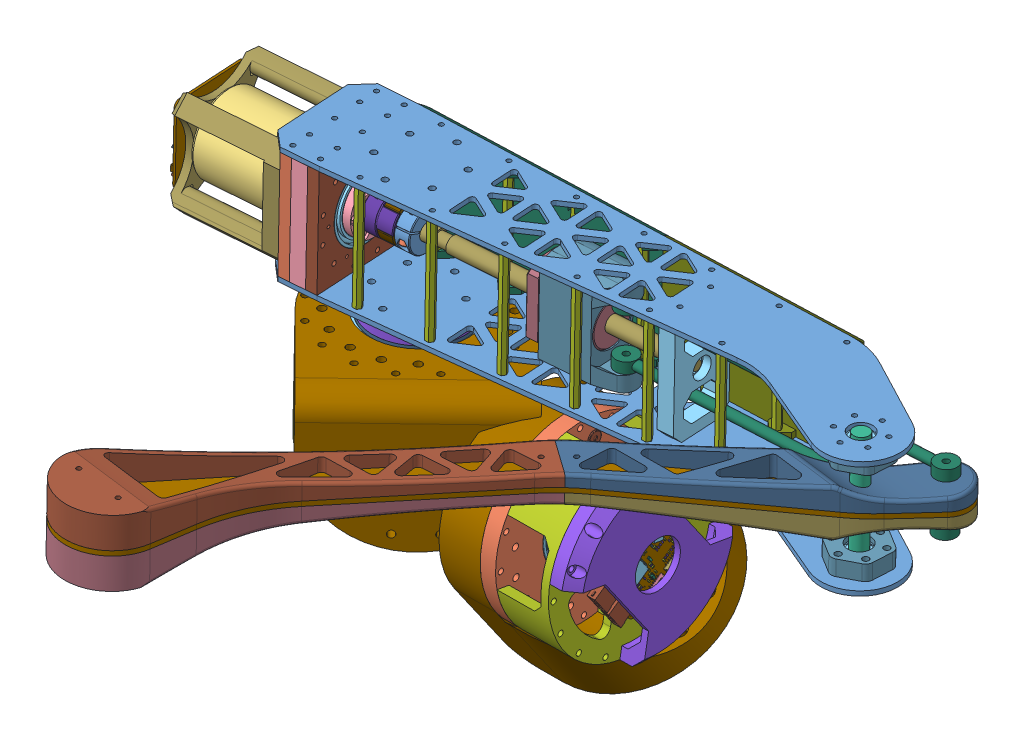
SolidWorks assembly Leg, configuration Default. Lengths in mm.
Overall size (497.03 260.49 419.34).
853 component instances, 131 part files, 94 mates.
Components (placement in the parent):
- Leg_Upper-1: Leg_Upper [Default] at (112.6903 199.4863 333.3624) x (0.999486 0.000829 0.03205) z (-0.03206 0.021084 0.999264) size (393.85 3 91.33)
- Cycloidal_5065-1: Cycloidal_5065 [Default] at (17.106 213.6076 395.5215) x (-0.000153 0.999777 -0.0211) z (-0.077938 -0.021048 -0.996736) size (81.75 102.59 81.75)
  - Motor_base_5065-1: Motor_base_5065 [Default] at (25.1788 43.6468 54.8039) size (70 7 70)
  - Flipsky 270kV motor.stp-1: Flipsky 270kV motor.stp [Default] at (25.1788 -19.3532 54.8039) x (0 1 0) z (-0.707107 0 0.707107) size (90.7 57.87 57.75)
  - Ring_pin_housing_5065-1: Ring_pin_housing_5065 [Default] at (25.1788 50.6468 54.8039) size (70 10 70)
  - radial ball bearing_68_iso-1: radial ball bearing_68_iso [ISO 15 RBB - 378 - 20,SI,NC,20_68] at (25.1788 45.3968 54.8039) x (0 1 0) z (0 0 1) size (3.5 12 12)
  - Ring_pin_5065-1: Ring_pin_5065 [Default] at (53.721 61.6863 58.0426) x (-1 0 0) z (0 0 1) size (13.84 14 13.84)
    - m2_pin-1: m2_pin [Default] at (4.7265 1.0395 10.5113) size (4 14 4)
    - Ball_bearing_4x10x4-1: Ball_bearing_4x10x4 [Default] at (4.7265 9.0395 10.5113) size (10 4 10)
    - Ball_bearing_4x10x4-2: Ball_bearing_4x10x4 [Default] at (4.7265 3.0395 10.5113) x (-0.837169 0 -0.546944) z (-0.546944 0 0.837169) size (10 4 10)
  - Ring_pin_5065-2: Ring_pin_5065 [Default] at (53.721 61.6863 30.5426) x (-1 0 0) z (0 0 1) size (13.84 14 13.84)
    - m2_pin-1: m2_pin [Default] at (4.7265 1.0395 10.5113) size (4 14 4)
    - Ball_bearing_4x10x4-1: Ball_bearing_4x10x4 [Default] at (4.7265 9.0395 10.5113) size (10 4 10)
    - Ball_bearing_4x10x4-2: Ball_bearing_4x10x4 [Default] at (4.7265 3.0395 10.5113) x (-0.837169 0 -0.546944) z (-0.546944 0 0.837169) size (10 4 10)
  - Ring_pin_5065-3: Ring_pin_5065 [Default] at (15.4727 61.6863 76.0894) x (-0.146403 0 0.989225) z (0.989225 0 0.146403) size (13.84 14 13.84)
    - m2_pin-1: m2_pin [Default] at (4.7265 1.0395 10.5113) size (4 14 4)
    - Ball_bearing_4x10x4-1: Ball_bearing_4x10x4 [Default] at (4.7265 9.0395 10.5113) size (10 4 10)
    - Ball_bearing_4x10x4-2: Ball_bearing_4x10x4 [Default] at (4.7265 3.0395 10.5113) x (-0.837169 0 -0.546944) z (-0.546944 0 0.837169) size (10 4 10)
  - Ring_pin_5065-4: Ring_pin_5065 [Default] at (6.0896 61.6863 58.0426) x (-1 0 0) z (0 0 1) size (13.84 14 13.84)
    - m2_pin-1: m2_pin [Default] at (4.7265 1.0395 10.5113) size (4 14 4)
    - Ball_bearing_4x10x4-1: Ball_bearing_4x10x4 [Default] at (4.7265 9.0395 10.5113) size (10 4 10)
    - Ball_bearing_4x10x4-2: Ball_bearing_4x10x4 [Default] at (4.7265 3.0395 10.5113) x (-0.837169 0 -0.546944) z (-0.546944 0 0.837169) size (10 4 10)
  - Ring_pin_5065-5: Ring_pin_5065 [Default] at (29.9053 61.6863 16.7926) x (-1 0 0) z (0 0 1) size (13.84 14 13.84)
    - m2_pin-1: m2_pin [Default] at (4.7265 1.0395 10.5113) size (4 14 4)
    - Ball_bearing_4x10x4-1: Ball_bearing_4x10x4 [Default] at (4.7265 9.0395 10.5113) size (10 4 10)
    - Ball_bearing_4x10x4-2: Ball_bearing_4x10x4 [Default] at (4.7265 3.0395 10.5113) x (-0.837169 0 -0.546944) z (-0.546944 0 0.837169) size (10 4 10)
  - Ring_pin_5065-6: Ring_pin_5065 [Default] at (6.0896 61.6863 30.5426) x (-1 0 0) z (0 0 1) size (13.84 14 13.84)
    - m2_pin-1: m2_pin [Default] at (4.7265 1.0395 10.5113) size (4 14 4)
    - Ball_bearing_4x10x4-1: Ball_bearing_4x10x4 [Default] at (4.7265 9.0395 10.5113) size (10 4 10)
    - Ball_bearing_4x10x4-2: Ball_bearing_4x10x4 [Default] at (4.7265 3.0395 10.5113) x (-0.837169 0 -0.546944) z (-0.546944 0 0.837169) size (10 4 10)
  - Eccentric_shaft_5065-1: Eccentric_shaft_5065 [Default] at (33.6841 47.0254 47.5733) x (0.059354 0 0.998237) z (-0.998237 0 0.059354) size (14 15 12)
    - Eccentric_shaft_bot_5065-1: Eccentric_shaft_bot_5065 [Default] at (6.713 3.6214 8.9195) size (12 5 12)
    - Eccentric_shaft_top_5065-1: Eccentric_shaft_top_5065 [Default] at (6.713 13.6214 8.9195) size (12 5 12)
    - Eccentric_shaft_bot_5065-2: Eccentric_shaft_bot_5065 [Default] at (6.713 8.6214 8.9195) x (-1 0 0) z (0 0 -1) size (12 5 12)
  - radial ball bearing_68_iso-2: radial ball bearing_68_iso [ISO 15 RBB - 1712 - 20,SI,NC,20_68] at (25.1788 63.6468 54.8039) x (0 1 0) z (0 0 1) size (4 18 18)
  - radial ball bearing_68_iso-3: radial ball bearing_68_iso [ISO 15 RBB - 1712 - 20,SI,NC,20_68] at (25.2381 58.6468 55.8021) x (0 -1 0) z (0.979554 0 -0.201181) size (4 18 18)
  - radial ball bearing_68_iso-4: radial ball bearing_68_iso [ISO 15 RBB - 1712 - 20,SI,NC,20_68] at (25.1194 53.6468 53.8056) x (0 1 0) z (0 0 1) size (4 18 18)
  - OutPut_shaft_5065-1: OutPut_shaft_5065 [Default] at (25.1788 60.6468 54.8039) x (0.014412 0 0.999896) z (-0.999896 0 0.014412) size (35 7 35)
  - Output_cover_5065-1: Output_cover_5065 [Default] at (25.1788 60.6468 54.8039) size (70 7 70)
  - Motor_cover_5065-1: Motor_cover_5065 [Default] at (25.1788 43.6468 54.8039) x (-1 0 0) z (0 0 1) size (70 70 70)
  - Cycloidal_discs_5065-3: Cycloidal_discs_5065 [Default] at (64.4697 27.0207 51.4124) x (-0.39126 0 0.92028) z (-0.92028 0 -0.39126) size (45.09 5 45.95)
    - Cycloidal_discs_5065-1: Cycloidal_discs_5065 [Default] at (17.5986 23.6261 35.277) size (45.09 5 45.95)
    - radial ball bearing_68_iso-1: radial ball bearing_68_iso [ISO 15 RBB - 274 - 14,SI,NC,14_68] at (10.5986 27.3761 23.1526) x (0 1 0) z (-0.544662 0 0.838655) size (2.5 7 7)
    - radial ball bearing_68_iso-2: radial ball bearing_68_iso [ISO 15 RBB - 274 - 14,SI,NC,14_68] at (24.5986 27.3761 23.1526) x (0 1 0) z (-0.544662 0 0.838655) size (2.5 7 7)
    - radial ball bearing_68_iso-3: radial ball bearing_68_iso [ISO 15 RBB - 274 - 14,SI,NC,14_68] at (31.5986 27.3761 35.277) x (0 1 0) z (-0.544662 0 0.838655) size (2.5 7 7)
    - radial ball bearing_68_iso-4: radial ball bearing_68_iso [ISO 15 RBB - 274 - 14,SI,NC,14_68] at (24.5986 27.3761 47.4013) x (0 1 0) z (-0.544662 0 0.838655) size (2.5 7 7)
    - radial ball bearing_68_iso-5: radial ball bearing_68_iso [ISO 15 RBB - 274 - 14,SI,NC,14_68] at (10.5986 27.3761 47.4013) x (0 1 0) z (-0.544662 0 0.838655) size (2.5 7 7)
    - radial ball bearing_68_iso-6: radial ball bearing_68_iso [ISO 15 RBB - 274 - 14,SI,NC,14_68] at (3.5986 27.3761 35.277) x (0 1 0) z (-0.544662 0 0.838655) size (2.5 7 7)
  - Cycloidal_discs_5065-5: Cycloidal_discs_5065 [Default] at (0.5658 32.0207 86.5503) x (-0.418554 0 -0.908192) z (0.908192 0 -0.418554) size (45.09 5 45.95)
    - Cycloidal_discs_5065-1: Cycloidal_discs_5065 [Default] at (17.5986 23.6261 35.277) size (45.09 5 45.95)
    - radial ball bearing_68_iso-1: radial ball bearing_68_iso [ISO 15 RBB - 274 - 14,SI,NC,14_68] at (10.5986 27.3761 23.1526) x (0 1 0) z (-0.544662 0 0.838655) size (2.5 7 7)
    - radial ball bearing_68_iso-2: radial ball bearing_68_iso [ISO 15 RBB - 274 - 14,SI,NC,14_68] at (24.5986 27.3761 23.1526) x (0 1 0) z (-0.544662 0 0.838655) size (2.5 7 7)
    - radial ball bearing_68_iso-3: radial ball bearing_68_iso [ISO 15 RBB - 274 - 14,SI,NC,14_68] at (31.5986 27.3761 35.277) x (0 1 0) z (-0.544662 0 0.838655) size (2.5 7 7)
    - radial ball bearing_68_iso-4: radial ball bearing_68_iso [ISO 15 RBB - 274 - 14,SI,NC,14_68] at (24.5986 27.3761 47.4013) x (0 1 0) z (-0.544662 0 0.838655) size (2.5 7 7)
    - radial ball bearing_68_iso-5: radial ball bearing_68_iso [ISO 15 RBB - 274 - 14,SI,NC,14_68] at (10.5986 27.3761 47.4013) x (0 1 0) z (-0.544662 0 0.838655) size (2.5 7 7)
    - radial ball bearing_68_iso-6: radial ball bearing_68_iso [ISO 15 RBB - 274 - 14,SI,NC,14_68] at (3.5986 27.3761 35.277) x (0 1 0) z (-0.544662 0 0.838655) size (2.5 7 7)
  - radial ball bearing_68_iso-5: radial ball bearing_68_iso [ISO 15 RBB - 274 - 14,SI,NC,14_68] at (25.1788 66.3968 54.8039) x (0 1 0) z (0 0 1) size (2.5 7 7)
  - foc-motor-controller.step-1: foc-motor-controller.step [Default] at (25.1788 -28.1532 54.8039) x (0 0 -1) z (0 -1 0) size (57.23 50 8.13)
    - RTA0040B.step-1: RTA0040B.step [Default] at (12.5014 -1.6986 1.595) x (-0.707107 -0.707107 0) z (0 0 1) size (6 6 1)
      - FRAME.step-1: FRAME.step [Default] x (1 0 0) z (0 -1 0) size (6 0.2 6)
        - SOLID.step-1: SOLID.step [Default] at origin size (0.4 0.2 0.22)
        - SOLID-0.step-1: SOLID-0.step [Default] at origin size (0.4 0.2 0.22)
        - SOLID-1.step-1: SOLID-1.step [Default] at origin size (0.4 0.2 0.22)
        - SOLID-2.step-1: SOLID-2.step [Default] at origin size (0.4 0.2 0.22)
        - SOLID-3.step-1: SOLID-3.step [Default] at origin size (0.4 0.2 0.22)
        - SOLID-4.step-1: SOLID-4.step [Default] at origin size (0.4 0.2 0.22)
        - SOLID-5.step-1: SOLID-5.step [Default] at origin size (0.4 0.2 0.22)
        - SOLID-6.step-1: SOLID-6.step [Default] at origin size (0.4 0.2 0.22)
        - SOLID-7.step-1: SOLID-7.step [Default] at origin size (0.4 0.2 0.22)
        - SOLID-8.step-1: SOLID-8.step [Default] at origin size (0.4 0.2 0.22)
        - SOLID-9.step-1: SOLID-9.step [Default] at origin size (0.22 0.2 0.4)
        - SOLID-10.step-1: SOLID-10.step [Default] at origin size (0.22 0.2 0.4)
        - SOLID-11.step-1: SOLID-11.step [Default] at origin size (0.22 0.2 0.4)
        - SOLID-12.step-1: SOLID-12.step [Default] at origin size (0.22 0.2 0.4)
        - SOLID-13.step-1: SOLID-13.step [Default] at origin size (0.22 0.2 0.4)
        - SOLID-14.step-1: SOLID-14.step [Default] at origin size (0.22 0.2 0.4)
        - SOLID-15.step-1: SOLID-15.step [Default] at origin size (0.22 0.2 0.4)
        - SOLID-16.step-1: SOLID-16.step [Default] at origin size (0.22 0.2 0.4)
        - SOLID-17.step-1: SOLID-17.step [Default] at origin size (4.15 0.2 4.15)
        - SOLID-18.step-1: SOLID-18.step [Default] at origin size (0.28 0.1 0.28)
        - SOLID-19.step-1: SOLID-19.step [Default] at origin size (0.28 0.1 0.28)
        - SOLID-20.step-1: SOLID-20.step [Default] at origin size (0.28 0.1 0.28)
        - SOLID-21.step-1: SOLID-21.step [Default] at origin size (0.28 0.1 0.28)
        - SOLID-22.step-1: SOLID-22.step [Default] at origin size (0.4 0.2 0.22)
        - SOLID-23.step-1: SOLID-23.step [Default] at origin size (0.4 0.2 0.22)
        - SOLID-24.step-1: SOLID-24.step [Default] at origin size (0.4 0.2 0.22)
        - SOLID-25.step-1: SOLID-25.step [Default] at origin size (0.4 0.2 0.22)
        - SOLID-26.step-1: SOLID-26.step [Default] at origin size (0.4 0.2 0.22)
        - SOLID-27.step-1: SOLID-27.step [Default] at origin size (0.4 0.2 0.22)
        - SOLID-28.step-1: SOLID-28.step [Default] at origin size (0.4 0.2 0.22)
        - SOLID-29.step-1: SOLID-29.step [Default] at origin size (0.4 0.2 0.22)
        - SOLID-30.step-1: SOLID-30.step [Default] at origin size (0.4 0.2 0.22)
        - SOLID-31.step-1: SOLID-31.step [Default] at origin size (0.4 0.2 0.22)
        - SOLID-32.step-1: SOLID-32.step [Default] at origin size (0.22 0.2 0.4)
        - SOLID-33.step-1: SOLID-33.step [Default] at origin size (0.22 0.2 0.4)
        - SOLID-34.step-1: SOLID-34.step [Default] at origin size (0.22 0.2 0.4)
        - SOLID-35.step-1: SOLID-35.step [Default] at origin size (0.22 0.2 0.4)
        - SOLID-36.step-1: SOLID-36.step [Default] at origin size (0.22 0.2 0.4)
        - SOLID-37.step-1: SOLID-37.step [Default] at origin size (0.22 0.2 0.4)
        - SOLID-38.step-1: SOLID-38.step [Default] at origin size (0.22 0.2 0.4)
        - SOLID-39.step-1: SOLID-39.step [Default] at origin size (0.22 0.2 0.4)
        - SOLID-40.step-1: SOLID-40.step [Default] at origin size (0.22 0.2 0.4)
        - SOLID-41.step-1: SOLID-41.step [Default] at origin size (0.22 0.2 0.4)
        - SOLID-42.step-1: SOLID-42.step [Default] at origin size (0.22 0.2 0.4)
        - SOLID-43.step-1: SOLID-43.step [Default] at origin size (0.22 0.2 0.4)
      - BODY.step-1: BODY.step [Default] at (0 0 0.025) x (1 0 0) z (0 -1 0) size (6 0.97 6)
    - Resonator_SMD_Murata_CSTxExxV-3Pin_3.0x1.1mm.step-1: Resonator_SMD_Murata_CSTxExxV-3Pin_3.0x1.1mm.step [Default] at (1.8 -7 1.595) x (0 1 0) z (0 0 1) size (3.2 1.35 0.9)
    - C_0603_1608Metric.step-1: C_0603_1608Metric.step [Default] at (6.2 -16.8 1.595) x (0 -1 0) z (0 0 1) size (1.6 0.8 0.8)
    - R_0603_1608Metric.step-1: R_0603_1608Metric.step [Default] at (11.8 -7.375 1.595) x (0 1 0) z (0 0 1) size (1.6 0.8 0.45)
    - R_0603_1608Metric.step-2: R_0603_1608Metric.step [Default] at (13.8 -16.8 1.595) x (0 1 0) z (0 0 1) size (1.6 0.8 0.45)
    - R_0603_1608Metric.step-3: R_0603_1608Metric.step [Default] at (18.1 -5.36 1.595) size (1.6 0.8 0.45)
    - C_0603_1608Metric.step-2: C_0603_1608Metric.step [Default] at (2.6 -0.5 1.595) x (0 -1 0) z (0 0 1) size (1.6 0.8 0.8)
    - R_0603_1608Metric.step-4: R_0603_1608Metric.step [Default] at (14.6 -11.3 1.595) x (0 1 0) z (0 0 1) size (1.6 0.8 0.45)
    - L_APV_ANR4020.step-1: L_APV_ANR4020.step [Default] at (22.3 -13.7 1.595) x (0 -1 0) z (0 0 1) size (4.02 4 2)
    - C_0603_1608Metric.step-3: C_0603_1608Metric.step [Default] at (0.3 -12.6 1.595) x (-1 0 0) z (0 0 1) size (1.6 0.8 0.8)
    - C_1206_3216Metric.step-1: C_1206_3216Metric.step [Default] at (15.7 11 1.595) x (0 1 0) z (0 0 1) size (3.2 1.6 1.6)
    - C_0603_1608Metric.step-4: C_0603_1608Metric.step [Default] at (0.3 -9.6 1.595) size (1.6 0.8 0.8)
    - R_0603_1608Metric.step-5: R_0603_1608Metric.step [Default] at (12.3 -16.8 1.595) x (0 1 0) z (0 0 1) size (1.6 0.8 0.45)
    - C_0603_1608Metric.step-5: C_0603_1608Metric.step [Default] at (-0.3 -16.6 1.595) x (0 1 0) z (0 0 1) size (1.6 0.8 0.8)
    - R_0603_1608Metric.step-6: R_0603_1608Metric.step [Default] at (10.9 4.1 1.595) size (1.6 0.8 0.45)
    - C_1206_3216Metric.step-2: C_1206_3216Metric.step [Default] at (6.3 11 1.595) x (0 1 0) z (0 0 1) size (3.2 1.6 1.6)
    - XT30PW_2_2_-M.G.B.step-1: XT30PW_2_2_-M.G.B.step [Default] at (-20.5 9.5 1.595) x (0 -1 0) z (-1 0 0) size (15.5 7.1 12.53)
    - R_0603_1608Metric.step-7: R_0603_1608Metric.step [Default] at (0.3 -11.1 1.595) size (1.6 0.8 0.45)
    - C_0603_1608Metric.step-6: C_0603_1608Metric.step [Default] at (19 -0.4 1.595) x (-0.707107 -0.707107 0) z (0 0 1) size (1.6 0.8 0.8)
    - C_1206_3216Metric.step-3: C_1206_3216Metric.step [Default] at (13.3 11 1.595) x (0 1 0) z (0 0 1) size (3.2 1.6 1.6)
    - R_0603_1608Metric.step-8: R_0603_1608Metric.step [Default] at (10.2 -7.375 1.595) x (0 -1 0) z (0 0 1) size (1.6 0.8 0.45)
    - JST_GH_SM08B-GHS-TB_1x08-1MP_P1.25mm_Horizontal.step-1: JST_GH_SM08B-GHS-TB_1x08-1MP_P1.25mm_Horizontal.step [Default] at (10 -22 1.595) size (13.25 4.95 4.25)
    - C_1206_3216Metric.step-4: C_1206_3216Metric.step [Default] at (-12.3 11 1.595) x (0 1 0) z (0 0 1) size (3.2 1.6 1.6)
    - JST_GH_SM06B-GHS-TB_1x06-1MP_P1.25mm_Horizontal.step-1: JST_GH_SM06B-GHS-TB_1x06-1MP_P1.25mm_Horizontal.step [Default] at (-4.3 -22 1.595) size (10.75 4.95 4.25)
    - C_0603_1608Metric.step-7: C_0603_1608Metric.step [Default] at (7.3 -4.5 1.595) x (-1 0 0) z (0 0 1) size (1.6 0.8 0.8)
    - R_0603_1608Metric.step-9: R_0603_1608Metric.step [Default] at (18.1 -3.86 1.595) x (-1 0 0) z (0 0 1) size (1.6 0.8 0.45)
    - C_1206_3216Metric.step-5: C_1206_3216Metric.step [Default] at (22.6794 -1.2206 1.595) x (0.707107 -0.707107 0) z (0 0 1) size (3.2 1.6 1.6)
    - R_Array_Convex_4x0402.step-1: R_Array_Convex_4x0402.step [Default] at (6.8 -2.5 1.595) size (1 2 0.35)
    - R_0603_1608Metric.step-10: R_0603_1608Metric.step [Default] at (7.7 -16.8 1.595) x (0 -1 0) z (0 0 1) size (1.6 0.8 0.45)
    - C_1206_3216Metric.step-6: C_1206_3216Metric.step [Default] at (8.7 11 1.595) x (0 1 0) z (0 0 1) size (3.2 1.6 1.6)
    - C_0603_1608Metric.step-8: C_0603_1608Metric.step [Default] at (16.1 -11.3 1.595) x (0 1 0) z (0 0 1) size (1.6 0.8 0.8)
    - SOT-23-5.step-1: SOT-23-5.step [Default] at (-3.1 -16.6 1.595) x (-1 0 0) z (0 0 1) size (2.8 2.9 1.55)
    - C_0603_1608Metric.step-9: C_0603_1608Metric.step [Default] at (17.8 -13.6 1.595) size (1.6 0.8 0.8)
    - R_0603_1608Metric.step-11: R_0603_1608Metric.step [Default] at (-11.5 -20.3875 1.595) x (0 -1 0) z (0 0 1) size (1.6 0.8 0.45)
    - C_0603_1608Metric.step-10: C_0603_1608Metric.step [Default] at (-12.4 2.3 1.595) x (0 1 0) z (0 0 1) size (1.6 0.8 0.8)
    - C_1206_3216Metric.step-7: C_1206_3216Metric.step [Default] at (18 11 1.595) x (0 1 0) z (0 0 1) size (3.2 1.6 1.6)
    - R_0603_1608Metric.step-12: R_0603_1608Metric.step [Default] at (-10.8105 -14.9971 1.595) x (-1 0 0) z (0 0 1) size (1.6 0.8 0.45)
    - C_0603_1608Metric.step-11: C_0603_1608Metric.step [Default] at (-13.8 -9.4 1.595) x (-1 0 0) z (0 0 1) size (1.6 0.8 0.8)
    - R_0603_1608Metric.step-13: R_0603_1608Metric.step [Default] at (-23.15 -14.5 1.595) x (-1 0 0) z (0 0 1) size (1.6 0.8 0.45)
    - C_0603_1608Metric.step-12: C_0603_1608Metric.step [Default] at (1.1 -0.2 1.595) x (0 1 0) z (0 0 1) size (1.6 0.8 0.8)
    - D_0805_2012Metric.step-1: D_0805_2012Metric.step [Default] at (22.9 -9.6 1.595) x (0 1 0) z (0 0 1) size (2 1.27 0.8)
    - C_0603_1608Metric.step-13: C_0603_1608Metric.step [Default] at (-7.8 3.775 1.595) x (0 -1 0) z (0 0 1) size (1.6 0.8 0.8)
    - R_0603_1608Metric.step-14: R_0603_1608Metric.step [Default] at (-6.4 -12.825 1.595) x (0 1 0) z (0 0 1) size (1.6 0.8 0.45)
    - L_0603_1608Metric.step-1: L_0603_1608Metric.step [Default] at (-10.1 3 1.595) size (1.6 0.8 0.8)
    - C_0603_1608Metric.step-14: C_0603_1608Metric.step [Default] at (17.9 0.7 1.595) x (-0.707107 -0.707107 0) z (0 0 1) size (1.6 0.8 0.8)
    - HVSSOP-10.step-1: HVSSOP-10.step [Default] at (18.6 -9.6 1.595) x (0 -1 0) z (-1 0 0) size (4.9 1.1 3)
    - C_0603_1608Metric.step-15: C_0603_1608Metric.step [Default] at (7.9 4.1 1.595) x (-1 0 0) z (0 0 1) size (1.6 0.8 0.8)
    - C_0603_1608Metric.step-16: C_0603_1608Metric.step [Default] at (21.1 -9.6 1.595) x (0 -1 0) z (0 0 1) size (1.6 0.8 0.8)
    - R_0603_1608Metric.step-15: R_0603_1608Metric.step [Default] at (-10.8105 -11.9971 1.595) x (-1 0 0) z (0 0 1) size (1.6 0.8 0.45)
    - R_0603_1608Metric.step-16: R_0603_1608Metric.step [Default] at (-18.2 -17.4 1.595) size (1.6 0.8 0.45)
    - C_1206_3216Metric.step-8: C_1206_3216Metric.step [Default] at (-3 11 1.595) x (0 1 0) z (0 0 1) size (3.2 1.6 1.6)
    - R_0603_1608Metric.step-17: R_0603_1608Metric.step [Default] at (-16.9 -20.4 1.595) x (0 -1 0) z (0 0 1) size (1.6 0.8 0.45)
    - R_0603_1608Metric.step-18: R_0603_1608Metric.step [Default] at (-13.3 -20.3875 1.595) x (0 -1 0) z (0 0 1) size (1.6 0.8 0.45)
    - R_0603_1608Metric.step-19: R_0603_1608Metric.step [Default] at (-15.1 -20.3875 1.595) x (0 -1 0) z (0 0 1) size (1.6 0.8 0.45)
    - C_0603_1608Metric.step-17: C_0603_1608Metric.step [Default] at (15.5 -14.4 1.595) x (0 -1 0) z (0 0 1) size (1.6 0.8 0.8)
    - LED_0603_1608Metric.step-1: LED_0603_1608Metric.step [Default] at (-11.5 -23.3875 1.595) x (0 1 0) z (0 0 1) size (1.6 0.8 1.1)
    - C_0805_2012Metric.step-1: C_0805_2012Metric.step [Default] at (19.95 -17 1.595) size (2 1.25 1.25)
    - D_SMB.step-1: D_SMB.step [Default] at (-16.5 11.208 1.595) x (0 -1 0) z (0 0 1) size (5.3 3.55 2.15)
    - C_1206_3216Metric.step-9: C_1206_3216Metric.step [Default] at (-5.3 11 1.595) x (0 1 0) z (0 0 1) size (3.2 1.6 1.6)
    - XT30PW_2_2_-M.G.B.step-2: XT30PW_2_2_-M.G.B.step [Default] at (-20.5 -6.5 1.595) x (0 -1 0) z (-1 0 0) size (15.5 7.1 12.53)
    - C_1206_3216Metric.step-10: C_1206_3216Metric.step [Default] at (1.7 11 1.595) x (0 1 0) z (0 0 1) size (3.2 1.6 1.6)
    - C_1206_3216Metric.step-11: C_1206_3216Metric.step [Default] at (11 11 1.595) x (0 1 0) z (0 0 1) size (3.2 1.6 1.6)
    - C_0603_1608Metric.step-18: C_0603_1608Metric.step [Default] at (-6.3 3.775 1.595) x (0 -1 0) z (0 0 1) size (1.6 0.8 0.8)
    - C_0603_1608Metric.step-19: C_0603_1608Metric.step [Default] at (16.8686 1.7314 1.595) x (0.707107 0.707107 0) z (0 0 1) size (1.6 0.8 0.8)
    - C_0603_1608Metric.step-20: C_0603_1608Metric.step [Default] at (-15.0105 -11.1 1.595) size (1.6 0.8 0.8)
    - C_1206_3216Metric.step-12: C_1206_3216Metric.step [Default] at (-7.7 11 1.595) x (0 1 0) z (0 0 1) size (3.2 1.6 1.6)
    - C_0603_1608Metric.step-21: C_0603_1608Metric.step [Default] at (-18.2 -15.8 1.595) size (1.6 0.8 0.8)
    - C_0603_1608Metric.step-22: C_0603_1608Metric.step [Default] at (-2.1 -11.3 1.595) x (0 -1 0) z (0 0 1) size (1.6 0.8 0.8)
    - C_0603_1608Metric.step-23: C_0603_1608Metric.step [Default] at (-10.8105 -13.4971 1.595) size (1.6 0.8 0.8)
    - C_1206_3216Metric.step-13: C_1206_3216Metric.step [Default] at (4 11 1.595) x (0 1 0) z (0 0 1) size (3.2 1.6 1.6)
    - R_0603_1608Metric.step-20: R_0603_1608Metric.step [Default] at (16 -17.8 1.595) x (0 1 0) z (0 0 1) size (1.6 0.8 0.45)
    - Texas_S-PVSON-N8.step-1: Texas_S-PVSON-N8.step [Default] at (-14.4105 -13.7 1.595) x (-1 0 0) z (0 0 1) size (3 2.98 0.92)
    - C_1206_3216Metric.step-14: C_1206_3216Metric.step [Default] at (21 -2.9 1.595) x (0.707107 -0.707107 0) z (0 0 1) size (3.2 1.6 1.6)
    - C_0603_1608Metric.step-24: C_0603_1608Metric.step [Default] at (-5.9 -16.6 1.595) x (0 1 0) z (0 0 1) size (1.6 0.8 0.8)
    - C_0603_1608Metric.step-25: C_0603_1608Metric.step [Default] at (-3.1 -14.1 1.595) size (1.6 0.8 0.8)
    - R_0603_1608Metric.step-21: R_0603_1608Metric.step [Default] at (7.2 -7.375 1.595) x (0 -1 0) z (0 0 1) size (1.6 0.8 0.45)
    - C_1206_3216Metric.step-15: C_1206_3216Metric.step [Default] at (-0.7 11 1.595) x (0 1 0) z (0 0 1) size (3.2 1.6 1.6)
    - LQFP-64_10x10mm_P0.5mm.step-1: LQFP-64_10x10mm_P0.5mm.step [Default] at (-7 -4.5 1.595) x (-1 0 0) z (0 0 1) size (12 12 1.5)
    - C_0805_2012Metric.step-2: C_0805_2012Metric.step [Default] at (23.35 -17 1.595) x (-1 0 0) z (0 0 1) size (2 1.25 1.25)
    - C_0603_1608Metric.step-26: C_0603_1608Metric.step [Default] at (10.8 -16.8 1.595) x (0 -1 0) z (0 0 1) size (1.6 0.8 0.8)
    - R_0603_1608Metric.step-22: R_0603_1608Metric.step [Default] at (17.5 -17.8 1.595) x (0 -1 0) z (0 0 1) size (1.6 0.8 0.45)
    - C_1206_3216Metric.step-16: C_1206_3216Metric.step [Default] at (20.3 11 1.595) x (0 1 0) z (0 0 1) size (3.2 1.6 1.6)
    - R_0603_1608Metric.step-23: R_0603_1608Metric.step [Default] at (9.2 -16.8 1.595) x (0 -1 0) z (0 0 1) size (1.6 0.8 0.45)
    - C_1206_3216Metric.step-17: C_1206_3216Metric.step [Default] at (-10 11 1.595) x (0 1 0) z (0 0 1) size (3.2 1.6 1.6)
    - R_0603_1608Metric.step-24: R_0603_1608Metric.step [Default] at (17.8 -15.2 1.595) size (1.6 0.8 0.45)
    - C_1206_3216Metric.step-18: C_1206_3216Metric.step [Default] at (19.9 2.6 1.595) x (-0.707107 0.707107 0) z (0 0 1) size (3.2 1.6 1.6)
    - C_0603_1608Metric.step-27: C_0603_1608Metric.step [Default] at (13.4 -7.375 1.595) x (0 -1 0) z (0 0 1) size (1.6 0.8 0.8)
    - R_0603_1608Metric.step-25: R_0603_1608Metric.step [Default] at (8.7 -7.375 1.595) x (0 -1 0) z (0 0 1) size (1.6 0.8 0.45)
    - PQFN-8-EP_6x5mm_P1.27mm_Generic.step-1: PQFN-8-EP_6x5mm_P1.27mm_Generic.step [Default] at (4.9 14.4 -0.085) x (0 1 0) z (0 0 -1) size (6.15 5.15 1.09)
    - C_0805_2012Metric.step-3: C_0805_2012Metric.step [Default] at (-3 8.9 -0.085) x (0 1 0) z (0 0 -1) size (2 1.25 1.25)
    - C_0603_1608Metric.step-28: C_0603_1608Metric.step [Default] at (1.5 -4.3 -0.085) x (0 1 0) z (0 0 -1) size (1.6 0.8 0.8)
    - R_2512_6332Metric.step-1: R_2512_6332Metric.step [Default] at (2.1 8.6 -0.085) x (-1 0 0) z (0 0 -1) size (6.3 3.2 0.6)
    - C_0805_2012Metric.step-4: C_0805_2012Metric.step [Default] at (18.8 8.9 -0.085) x (0 1 0) z (0 0 -1) size (2 1.25 1.25)
    - C_0805_2012Metric.step-5: C_0805_2012Metric.step [Default] at (-5.2 8.901 -0.085) x (0 1 0) z (0 0 -1) size (2 1.25 1.25)
    - PQFN-8-EP_6x5mm_P1.27mm_Generic.step-2: PQFN-8-EP_6x5mm_P1.27mm_Generic.step [Default] at (16.9 14.6 -0.085) x (0 -1 0) z (0 0 -1) size (6.15 5.15 1.09)
    - PQFN-8-EP_6x5mm_P1.27mm_Generic.step-3: PQFN-8-EP_6x5mm_P1.27mm_Generic.step [Default] at (-1.1 14.6 -0.085) x (0 -1 0) z (0 0 -1) size (6.15 5.15 1.09)
    - R_0603_1608Metric.step-26: R_0603_1608Metric.step [Default] at (8.2 8.8 -0.085) x (0 1 0) z (0 0 -1) size (1.6 0.8 0.45)
    - R_2512_6332Metric.step-2: R_2512_6332Metric.step [Default] at (-10.3 8.601 -0.085) x (1 0 0) z (0 0 -1) size (6.3 3.2 0.6)
    - TSSOP-16_4.4x5mm_P0.65mm.step-1: TSSOP-16_4.4x5mm_P0.65mm.step [Default] at (0 0 -0.085) x (-1 0 0) z (0 0 -1) size (6.4 5 1.1)
    - C_0603_1608Metric.step-29: C_0603_1608Metric.step [Default] at (0 -4.25 -0.085) x (0 1 0) z (0 0 -1) size (1.6 0.8 0.8)
    - PQFN-8-EP_6x5mm_P1.27mm_Generic.step-4: PQFN-8-EP_6x5mm_P1.27mm_Generic.step [Default] at (10.9 14.4 -0.085) x (0 1 0) z (0 0 -1) size (6.15 5.15 1.09)
    - R_2512_6332Metric.step-3: R_2512_6332Metric.step [Default] at (13.7 8.6 -0.085) x (1 0 0) z (0 0 -1) size (6.3 3.2 0.6)
    - PQFN-8-EP_6x5mm_P1.27mm_Generic.step-5: PQFN-8-EP_6x5mm_P1.27mm_Generic.step [Default] at (-13.1 14.401 -0.085) x (0 1 0) z (0 0 -1) size (6.15 5.15 1.09)
    - C_0603_1608Metric.step-30: C_0603_1608Metric.step [Default] at (-1.5 -4.3 -0.085) x (0 -1 0) z (0 0 -1) size (1.6 0.8 0.8)
    - PQFN-8-EP_6x5mm_P1.27mm_Generic.step-6: PQFN-8-EP_6x5mm_P1.27mm_Generic.step [Default] at (-7.1 14.601 -0.085) x (0 -1 0) z (0 0 -1) size (6.15 5.15 1.09)
    - foc-motor-controller_PCB.step-1: foc-motor-controller_PCB.step [Default] at origin size (50 50 1.51)
  - hex thin nut chamfered gradeab_iso-1: hex thin nut chamfered gradeab_iso [PreviewCfg] at (46.6788 -26.3532 33.3039) x (0.517651 0 -0.855592) z (0 1 0) size (5.5 6.35 1.8)
  - m3_5065-1: m3_5065 [Default] at (11.1802 50.6468 55.0056) size (3 17 3)
  - radial ball bearing_68_iso-7: radial ball bearing_68_iso [ISO 15 RBB - 1835 - 28,SI,NC,28_68] at (25.1788 64.1468 54.8039) x (0 1 0) z (0 0 1) size (7 47 47)
- Leg_Upper-2: Leg_Upper [Default] at (112.6792 272.4701 331.8221) x (0.999486 0.000829 0.03205) z (-0.03206 0.021084 0.999264) size (393.85 3 91.33)
- ball_screw-1: ball_screw [Default] at (132.8116 237.4478 330.9874) x (0.073294 0.357923 0.93087) z (-0.026502 0.93375 -0.356944) size (10 178 10)
- ball_screw_slider-1: ball_screw_slider [Default] at (198.3229 237.3497 325.867) x (0.000153 -0.999777 0.0211) z (0.077938 0.021048 0.996736) size (45 40.01 30)
- connection_rod_base-1: connection_rod_base [Default] at (198.3229 237.3497 325.867) x (0.000153 -0.999777 0.0211) z (0.077938 0.021048 0.996736) size (61.15 47.98 30)
- Link_Rod-1: Link_Rod [Default] at (239.1962 250.2857 322.3978) x (0.998607 -0.00096 -0.05275) z (0.052759 0.021079 0.998385) size (214 7 14)
- Link_Rod-2: Link_Rod [Default] at (239.2012 217.293 323.0941) x (0.998607 -0.00096 -0.05275) z (0.052759 0.021079 0.998385) size (214 7 14)
- Shaft Coupler D25L30 8x8.step-1: Shaft Coupler D25L30 8x8.step [Default] at (126.1016 219.0711 339.3901) x (-0.029261 0.919514 -0.391966) z (0.996958 -0.001492 -0.077924) size (25 25 30)
  - 8x8_Flexible_Spider_Shaft_Coupling.step-1: 8x8_Flexible_Spider_Shaft_Coupling.step [Default] at origin size (25 25 30)
    - Screw.step-1: Screw.step [Default] at (-0.1468 24 -24) size (5.4 14.9 5.4)
    - Coupler R.step-1: Coupler R.step [Default] at origin size (25 25 20)
    - Plastic.step-1: Plastic.step [Default] at (-0.0052 0 -14) size (21.45 21.45 11)
    - Coupler L.step-1: Coupler L.step [Default] at (-0.0052 0.0052 -24) size (25 25 20)
    - Screw (1).step-1: Screw (1).step [Default] at (30.9948 0.0052 -24) size (14.9 5.4 5.4)
- m8-1: m8 [Default] at (86.951 237.5191 334.5651) x (-0.049546 0.759651 -0.64844) z (0.060162 0.650329 0.757267) size (15.01 18.7 13)
- Output_Shaft_holder-1: Output_Shaft_holder [Default] at (80.2719 237.5264 335.094) x (-0.067006 0.494241 -0.866739) z (-0.039806 -0.869324 -0.492638) size (35 5 35)
- ball_screw_holder-1: ball_screw_holder [Default] at (285.3462 237.2195 319.0651) x (0.000153 -0.999777 0.0211) z (-0.077938 -0.021048 -0.996736) size (70 10 40)
- radial ball bearing_68_iso-1: radial ball bearing_68_iso [ISO 15 RBB - 286 - 10,SI,NC,10_68] at (277.869 237.2307 319.6495) x (0.996958 -0.001492 -0.077924) z (0.054373 0.729627 0.68168) size (5 13 13)
- m10-1: m10 [Default] at (412.5361 199.7352 342.9773) x (1 0.000153 -0.000002) z (-0.000002 0.0211 0.999777) size (10 76 10)
- radial ball bearing_68_iso-3: radial ball bearing_68_iso [ISO 15 RBB - 1910 - 10,SI,NC,10_68] at (412.5352 205.7338 342.8507) x (-0.000153 0.999777 -0.0211) z (-0.450103 0.018773 0.892779) size (6 22 22)
- radial ball bearing_68_iso-4: radial ball bearing_68_iso [ISO 15 RBB - 1910 - 10,SI,NC,10_68] at (412.5254 269.7196 341.5003) x (-0.000153 0.999777 -0.0211) z (-0.985774 0.003396 0.168044) size (6 22 22)
- brass_spacer_70mm-1: brass_spacer_70mm [Default] at (140.9108 201.8627 303.5749) x (0.999323 -0.000623 -0.036773) z (0.036778 0.021091 0.999101) size (5.31 70 4.6)
- brass_spacer_70mm-2: brass_spacer_70mm [Default] at (97.9401 201.8896 305.1625) x (0.467811 -0.018577 -0.883633) z (0.883828 0.010006 0.467704) size (5.31 70 4.6)
- brass_spacer_70mm-3: brass_spacer_70mm [Default] at (269.8228 201.7819 298.8123) x (0.999323 -0.000623 -0.036773) z (0.036778 0.021091 0.999101) size (5.31 70 4.6)
- brass_spacer_70mm-4: brass_spacer_70mm [Default] at (226.8521 201.8088 300.3998) x (0.531512 0.017954 0.84686) z (-0.847051 0.011085 0.531397) size (5.31 70 4.6)
- brass_spacer_70mm-5: brass_spacer_70mm [Default] at (183.8815 201.8357 301.9874) x (0.999323 -0.000623 -0.036773) z (0.036778 0.021091 0.999101) size (5.31 70 4.6)
- brass_spacer_70mm-6: brass_spacer_70mm [Default] at (355.7642 201.728 295.6372) x (0.999323 -0.000623 -0.036773) z (0.036778 0.021091 0.999101) size (5.31 70 4.6)
- brass_spacer_70mm-7: brass_spacer_70mm [Default] at (312.7935 201.755 297.2247) x (-0.999323 0.000623 0.036773) z (-0.036778 -0.021091 -0.999101) size (5.31 70 4.6)
- brass_spacer_70mm-8: brass_spacer_70mm [Default] at (273.3105 202.7202 343.2485) x (1 0.000153 -0.000002) z (-0.000002 0.0211 0.999777) size (5.31 70 4.6)
- brass_spacer_70mm-9: brass_spacer_70mm [Default] at (230.6055 202.8198 348.2762) x (1 0.000153 -0.000002) z (-0.000002 0.0211 0.999777) size (5.31 70 4.6)
- brass_spacer_70mm-10: brass_spacer_70mm [Default] at (316.0154 202.6207 338.2207) x (1 0.000153 -0.000002) z (-0.000002 0.0211 0.999777) size (5.31 70 4.6)
- brass_spacer_70mm-11: brass_spacer_70mm [Default] at (187.9006 202.9194 353.304) x (1 0.000153 -0.000002) z (-0.000002 0.0211 0.999777) size (5.31 70 4.6)
- brass_spacer_70mm-12: brass_spacer_70mm [Default] at (102.4907 203.1185 363.3595) x (1 0.000153 -0.000002) z (-0.000002 0.0211 0.999777) size (5.31 70 4.6)
- brass_spacer_70mm-13: brass_spacer_70mm [Default] at (145.1957 203.0189 358.3317) x (-0.516003 0.017995 0.856398) z (-0.856587 -0.011019 -0.515886) size (5.31 70 4.6)
- Output_2-1: Output_2 [Default] at (112.6906 191.4881 333.5311) x (0.999485 0.00083 0.032093) z (-0.032103 0.021084 0.999262) size (60 8 60)
- Output_2-2: Output_2 [Default] at (193.6649 124.5302 333.9109) x (0.000086 -0.999787 0.020658) z (-0.007648 -0.020658 -0.999757) size (60 8 60)
- Leg_Lower-1: Leg_Lower [Default] at (-80.3784 36.3685 402.6789) x (0.659733 -0.015756 -0.751335) z (0.7515 0.014035 0.659583) size (435 46.43 76.27)
  - Leg_Lower_in-1: Leg_Lower_in [Default] at (367.4739 202.5146 333.3401) size (435 3 72.6)
  - Leg_Lower_out_left_1-1: Leg_Lower_out_left_1 [Default] at (367.4739 204.0146 333.3401) size (195.32 15.92 59)
  - Leg_Lower_out_left_2-1: Leg_Lower_out_left_2 [Default] at (367.4739 204.0146 333.3401) size (243.01 21.71 76.27)
  - MirrorLeg_Lower_out_left_1-2: MirrorLeg_Lower_out_left_1 [Default] at (367.4739 201.0146 333.3401) x (1 0 0) z (0 0 -1) size (195.32 15.92 59)
  - MirrorLeg_Lower_out_left_2-2: MirrorLeg_Lower_out_left_2 [Default] at (367.4739 201.0146 333.3401) x (1 0 0) z (0 0 -1) size (243.01 21.71 76.27)
- bearing_knee_holder-2: bearing_knee_holder [Default] at (412.5357 202.7345 342.914) x (0.999486 0.000829 0.03205) z (-0.03206 0.021084 0.999264) size (32 10 35.4)
- bearing_knee_holder-3: bearing_knee_holder [Default] at (412.5249 272.7189 341.437) x (-0.527508 0.017845 0.849363) z (0.84955 0.01126 0.527388) size (32 10 35.4)
